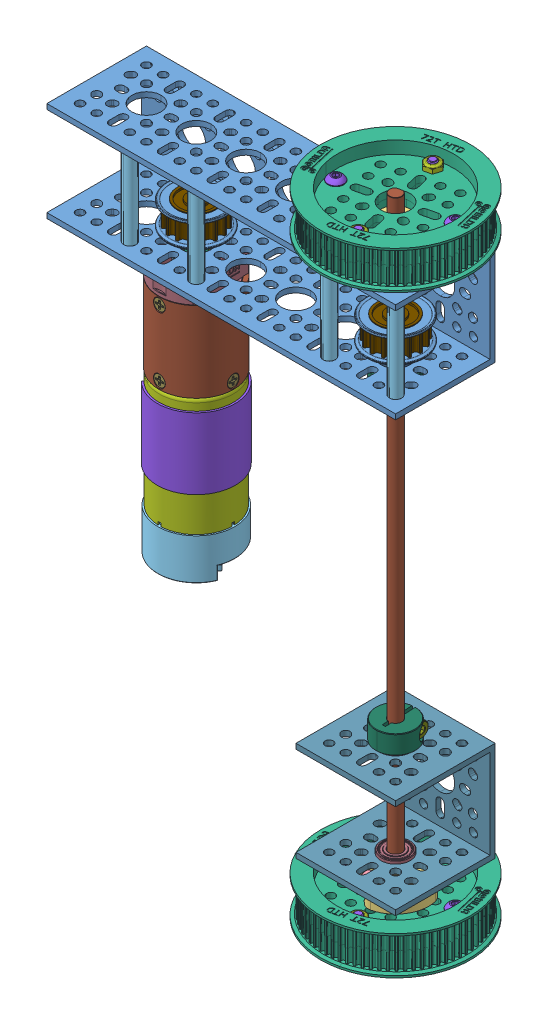
SolidWorks assembly motorisationElevateur, configuration Défaut. Lengths in mm.
Overall size (187.17 304.42 86.33).
106 component instances, 34 part files, 50 mates.
Components (placement in the parent):
- 1120-0006-0168 channel-1: 1120-0006-0168 channel [Défaut] at (77.0358 3.4821 146.5) x (0 -1 0) z (0 0 -1) size (48 168 48)
- 5202-2402-0051 moteur-1: 5202-2402-0051 moteur [Défaut] at (-54.0426 -130.9533 205.1707) x (0 0 1) z (-1 0 0) size (52.36 150.75 52.36)
  - 5202-2402-0051.step-1: 5202-2402-0051.step [Défaut] at origin size (52.36 150.75 52.36)
    - 5000-0002-0001.step-1: 5000-0002-0001.step [Défaut] at origin size (52.36 88.75 52.36)
      - 5000-0002-0001 encoder cap.step-1: 5000-0002-0001 encoder cap.step [Défaut] x (0 1 0) z (0 0 1) size (22.84 52.33 52.33)
        - JST-XH-4POS-VERT (1).step-1: JST-XH-4POS-VERT (1).step [Défaut] at (2.8 12.25 -75.95) x (1 0 0) z (0 0 -1) size (10.4 12.83 12.83)
          - Plastic (1).step-1: Plastic (1).step [Défaut] at (-6.1146 -33.6358 -52.1967) x (0 0.707107 0.707107) z (-1 0 0) size (12.4 5.75 7)
          - Pin (1).step-1: Pin (1).step [Défaut] at (-7.7146 -29.3225 -51.2067) x (0 0.707107 0.707107) z (-1 0 0) size (0.64 0.64 10)
          - Pin (1).step-2: Pin (1).step [Défaut] at (-7.7146 -34.6258 -56.51) x (0 0.707107 0.707107) z (-1 0 0) size (0.64 0.64 10)
          - Pin (1).step-3: Pin (1).step [Défaut] at (-7.7146 -32.858 -54.7423) x (0 0.707107 0.707107) z (-1 0 0) size (0.64 0.64 10)
          - Pin (1).step-4: Pin (1).step [Défaut] at (-7.7146 -31.0902 -52.9745) x (0 0.707107 0.707107) z (-1 0 0) size (0.64 0.64 10)
        - screw.step-1: screw.step [Défaut] at (-41.264 -8.1646 3.9905) x (0.882398 0 0.470504) z (0 -1 0) size (8.86 7.85 4.95)
          - 99461A915_Phillips Rounded Head Thread-Forming Screws (1).step-1: 99461A915_Phillips Rounded Head Thread-Forming Screws (1).step [Défaut] at (27.264 -14.6475 -49.347) x (-0.332697 -0.623949 0.707107) z (-0.882398 0.470504 0) size (3.5 3.5 7.4)
        - screw_1.step-1: screw_1.step [Défaut] at (-14.4172 7.3354 3.9905) x (0.882398 0 0.470504) z (0 -1 0) size (8.86 7.85 4.95)
          - 99461A915_Phillips Rounded Head Thread-Forming Screws (1).step-1: 99461A915_Phillips Rounded Head Thread-Forming Screws (1).step [Défaut] at (-10.5142 -28.4382 -25.8237) x (-0.332697 -0.623949 0.707107) z (-0.882398 0.470504 0) size (3.5 3.5 7.4)
        - endcap.step-1: endcap.step [Défaut] at (72.6354 37.1707 -11.0784) x (0 -0.707107 -0.707107) z (1 0 0) size (37 37 21.84)
        - base.step-1: base.step [Défaut] at (-55.8646 37.1707 -11.0784) x (0 -0.707107 -0.707107) z (-1 0 0) size (34.96 34.31 1)
      - 5000-0002-0001 body.step-1: 5000-0002-0001 body.step [Défaut] at (-37.1707 3.4854 -11.0784) size (35.61 61.8 35.61)
      - 5000-0002-0001 motor shield.step-1: 5000-0002-0001 motor shield.step [Défaut] at (-37.1707 54.6354 -11.0784) x (0.808104 0 -0.58904) z (0 -1 0) size (37.5 37.27 34.15)
      - 5000-0002-0001 motor shaft.step-1: 5000-0002-0001 motor shaft.step [Défaut] at (-37.1707 59.4854 -11.0784) size (3.14 12.45 3.14)
    - 5102-0024-0051.step-1: 5102-0024-0051.step [Défaut] at origin size (36 76.68 35.98)
      - 5102 Gearbox Base.step-1: 5102 Gearbox Base.step [Défaut] at (-37.1707 60.1354 -11.0784) size (31.91 5.69 31.91)
      - 5102 Gearbox Barrel (3 stage, simple)_Gear Blank.step-1: 5102 Gearbox Barrel (3 stage, simple)_Gear Blank.step [Défaut] at (-37.1707 111.8354 -11.0784) x (1 0 0) z (0 -1 0) size (35.98 35.98 38.7)
      - 5102 Gearbox Barrel Screw (M3 x 8mm length Flat Head)_92010A118.step-1: 5102 Gearbox Barrel Screw (M3 x 8mm length Flat Head)_92010A118.step [Défaut] at (-37.1707 63.6354 5.0046) x (0.002439 -0.999997 0) z (0 0 1) size (5.46 5.46 8)
      - 5102 Gearbox Face.step-1: 5102 Gearbox Face.step [Défaut] at (-37.1707 93.3354 -11.0784) size (36 17.1 31.91)
      - 5102 Gearbox Bearing.step-1: 5102 Gearbox Bearing.step [Défaut] at (-37.1707 101.4354 -11.0784) size (17 5 17)
      - 5102 Gearbox Shaft (23.5mm Length, Simple).step-1: 5102 Gearbox Shaft (23.5mm Length, Simple).step [Défaut] at (-37.1707 89.9754 -11.0784) x (0.894773 0 -0.44652) z (0.44652 0 0.894773) size (8.97 40.6 8.97)
      - 5102 Gearbox Snap Ring.step-1: 5102 Gearbox Snap Ring.step [Défaut] at (-37.1707 106.5104 -11.0784) x (0 1 0) z (0 0 1) size (0.85 13.06 10.66)
      - 5102 Gearbox Barrel Screw (M3 x 8mm length Flat Head)_92010A118.step-2: 5102 Gearbox Barrel Screw (M3 x 8mm length Flat Head)_92010A118.step [Défaut] at (-37.1707 95.3354 5.0046) x (-0.002439 -0.999997 0) z (0 0 1) size (5.46 5.46 8)
      - 5102 Gearbox Barrel Screw (M3 x 8mm length Flat Head)_92010A118.step-3: 5102 Gearbox Barrel Screw (M3 x 8mm length Flat Head)_92010A118.step [Défaut] at (-21.0877 63.6354 -11.0784) x (0 -0.999997 -0.002439) z (1 0 0) size (5.46 5.46 8)
      - 5102 Gearbox Barrel Screw (M3 x 8mm length Flat Head)_92010A118.step-4: 5102 Gearbox Barrel Screw (M3 x 8mm length Flat Head)_92010A118.step [Défaut] at (-37.1707 63.6354 -27.1614) x (-0.002439 -0.999997 0) z (0 0 -1) size (5.46 5.46 8)
      - 5102 Gearbox Barrel Screw (M3 x 8mm length Flat Head)_92010A118.step-5: 5102 Gearbox Barrel Screw (M3 x 8mm length Flat Head)_92010A118.step [Défaut] at (-53.2537 63.6354 -11.0784) x (0 -0.999997 0.002439) z (-1 0 0) size (5.46 5.46 8)
      - 5102 Gearbox Barrel Screw (M3 x 8mm length Flat Head)_92010A118.step-6: 5102 Gearbox Barrel Screw (M3 x 8mm length Flat Head)_92010A118.step [Défaut] at (-21.0877 95.3354 -11.0784) x (0 -0.999997 0.002439) z (1 0 0) size (5.46 5.46 8)
      - 5102 Gearbox Barrel Screw (M3 x 8mm length Flat Head)_92010A118.step-7: 5102 Gearbox Barrel Screw (M3 x 8mm length Flat Head)_92010A118.step [Défaut] at (-37.1707 95.3354 -27.1614) x (0.002439 -0.999997 0) z (0 0 -1) size (5.46 5.46 8)
      - 5102 Gearbox Barrel Screw (M3 x 8mm length Flat Head)_92010A118.step-8: 5102 Gearbox Barrel Screw (M3 x 8mm length Flat Head)_92010A118.step [Défaut] at (-53.2537 95.3354 -11.0784) x (0 -0.999997 -0.002439) z (-1 0 0) size (5.46 5.46 8)
      - 5102 Gearbox Bearing.step-2: 5102 Gearbox Bearing.step [Défaut] at (-37.1707 93.3354 -11.0784) size (17 5 17)
      - 5102 Gearbox Base Mounting Screw M3 x 5mm length SHCS)_91290A110.step-1: 5102 Gearbox Base Mounting Screw M3 x 5mm length SHCS)_91290A110.step [Défaut] at (-46.0096 57.2554 -2.2396) x (0.056382 0 0.998409) z (0 -1 0) size (5.5 5.5 8)
      - 5102 Gearbox Base Mounting Screw M3 x 5mm length SHCS)_91290A110.step-2: 5102 Gearbox Base Mounting Screw M3 x 5mm length SHCS)_91290A110.step [Défaut] at (-28.3319 57.2554 -2.2396) x (0.998409 0 -0.056382) z (0 -1 0) size (5.5 5.5 8)
      - 5102 Gearbox Base Mounting Screw M3 x 5mm length SHCS)_91290A110.step-3: 5102 Gearbox Base Mounting Screw M3 x 5mm length SHCS)_91290A110.step [Défaut] at (-28.3319 57.2554 -19.9173) x (-0.056382 0 -0.998409) z (0 -1 0) size (5.5 5.5 8)
      - 5102 Gearbox Base Mounting Screw M3 x 5mm length SHCS)_91290A110.step-4: 5102 Gearbox Base Mounting Screw M3 x 5mm length SHCS)_91290A110.step [Défaut] at (-46.0096 57.2554 -19.9173) x (-0.998409 0 0.056382) z (0 -1 0) size (5.5 5.5 8)
- 3417-1006-0016 assembly pulley-1: 3417-1006-0016 assembly pulley [Défaut] at (-65.9677 49.45 158.6429) x (0 1 0) z (1 0 0) size (12.01 27.98 27.98)
  - 3417-1006-0016 assembly.STEP-1: 3417-1006-0016 assembly.STEP [Défaut] at origin size (12.01 27.98 27.98)
    - 3417-1006-0016 body.STEP-1: 3417-1006-0016 body.STEP [Défaut] at (-62.7232 -4.1348 4.7756) size (12 23.97 23.97)
    - 3417-1006-0016 ring.STEP-1: 3417-1006-0016 ring.STEP [Défaut] at (-50.8429 9.3571 23.0035) x (0 -1 0) z (0 0 1) size (27.98 1.38 27.98)
    - 3417-1006-0016 ring.STEP-2: 3417-1006-0016 ring.STEP [Défaut] at (-60.0929 9.3571 23.0035) x (0 -1 0) z (0 0 -1) size (27.98 1.38 27.98)
    - 2806-0005-0006_91390A118.STEP-1: 2806-0005-0006_91390A118.STEP [Défaut] at (-55.4679 9.3571 17.1119) x (-0.607877 0.794031 0) z (0 0 -1) size (5.01 5.01 6.01)
- 3417-1006-0016 assembly pulley-2: 3417-1006-0016 assembly pulley [Défaut] at (56.9629 49.45 143.4787) x (0 1 0) z (0.225568 0 0.974227) size (12.01 27.98 27.98)
  - 3417-1006-0016 assembly.STEP-1: 3417-1006-0016 assembly.STEP [Défaut] at origin size (12.01 27.98 27.98)
    - 3417-1006-0016 body.STEP-1: 3417-1006-0016 body.STEP [Défaut] at (-62.7232 -4.1348 4.7756) size (12 23.97 23.97)
    - 3417-1006-0016 ring.STEP-1: 3417-1006-0016 ring.STEP [Défaut] at (-50.8429 9.3571 23.0035) x (0 -1 0) z (0 0 1) size (27.98 1.38 27.98)
    - 3417-1006-0016 ring.STEP-2: 3417-1006-0016 ring.STEP [Défaut] at (-60.0929 9.3571 23.0035) x (0 -1 0) z (0 0 -1) size (27.98 1.38 27.98)
    - 2806-0005-0006_91390A118.STEP-1: 2806-0005-0006_91390A118.STEP [Défaut] at (-55.4679 9.3571 17.1119) x (-0.607877 0.794031 0) z (0 0 -1) size (5.01 5.01 6.01)
- 1309-0016-1006 assembly-1: 1309-0016-1006 assembly [Défaut] at (37.2879 44.7557 158.8543) x (-0.848383 0 -0.529382) z (0 -1 0) size (28.36 32 10.95)
  - 1309-0016-1006 assembly.STEP-1: 1309-0016-1006 assembly.STEP [Défaut] at origin size (28.36 32 10.95)
    - 1309-0016-1006.STEP-1: 1309-0016-1006.STEP [Défaut] at (-18.2019 0.5776 8.7736) size (25.38 32 10)
    - 2800-0004-0014_90128A207.STEP-1: 2800-0004-0014_90128A207.STEP [Défaut] at (-16.149 11.6963 8.7736) x (0.5 -0.5 -0.707107) z (0.707107 0.707107 0) size (7 7 18.01)
    - 2800-0004-0014_90128A207.STEP-2: 2800-0004-0014_90128A207.STEP [Défaut] at (-20.2547 -10.5411 8.7736) x (-0.5 0.5 -0.707107) z (-0.707107 -0.707107 0) size (7 7 18.01)
- 1501-0006-0430 renfort-1: 1501-0006-0430 renfort [Défaut] at (69.0358 3.4821 184) size (5.95 43.01 5.95)
- 1501-0006-0430 renfort-2: 1501-0006-0430 renfort [Défaut] at (37.0358 3.4821 184) size (5.95 43.01 5.95)
- 1501-0006-0430 renfort-3: 1501-0006-0430 renfort [Défaut] at (-26.9642 3.4821 184) size (5.95 43.01 5.95)
- 1501-0006-0430 renfort-4: 1501-0006-0430 renfort [Défaut] at (-58.9642 3.4821 184) size (5.95 43.01 5.95)
- 3402-0014-0072 pulley-1: 3402-0014-0072 pulley [Défaut] at (-4.0352 74.1976 188.4845) x (-0.974227 0 0.225568) z (0 -1 0) size (71.96 71.96 18.5)
  - 3402-0014-0072 assembly.STEP-1: 3402-0014-0072 assembly.STEP [Défaut] at origin size (71.96 71.96 18.5)
    - 3402-0014-0072.STEP-1: 3402-0014-0072.STEP [Défaut] at (-60.2208 7.0832 38.7155) size (71.96 71.96 10.5)
    - 3402-0014-0072.STEP-2: 3402-0014-0072.STEP [Défaut] at (-60.2208 7.0832 23.2155) x (0 -1 0) z (0 0 -1) size (71.96 71.96 10.5)
    - 2812-0004-0007_90576A103.STEP-1: 2812-0004-0007_90576A103.STEP [Défaut] at (-60.2208 31.0832 29.7155) x (0.866025 0.5 0) z (-0.5 0.866025 0) size (7.02 4.86 8.1)
    - 2812-0004-0007_90576A103.STEP-2: 2812-0004-0007_90576A103.STEP [Défaut] at (-60.2208 -16.9168 29.7155) x (0 1 0) z (-1 0 0) size (7.02 4.86 8.1)
    - 2812-0004-0007_90576A103.STEP-3: 2812-0004-0007_90576A103.STEP [Défaut] at (-84.2208 7.0832 32.2155) x (0.5 0.866025 0) z (0.866025 -0.5 0) size (7.02 4.86 8.1)
    - 2812-0004-0007_90576A103.STEP-4: 2812-0004-0007_90576A103.STEP [Défaut] at (-36.2208 7.0832 32.2155) x (1 0 0) z (0 -1 0) size (7.02 4.86 8.1)
    - 2802-0004-0010_92095A480.STEP-1: 2802-0004-0010_92095A480.STEP [Défaut] at (-36.2208 7.0832 25.5155) x (-0.923728 -0.383049 0) z (0 0 -1) size (13.53 12.99 15.57)
    - 2802-0004-0010_92095A480.STEP-2: 2802-0004-0010_92095A480.STEP [Défaut] at (-84.2208 7.0832 25.5155) x (0.923728 0.383049 0) z (0 0 -1) size (13.53 12.99 15.57)
    - 2802-0004-0010_92095A480.STEP-3: 2802-0004-0010_92095A480.STEP [Défaut] at (-60.2208 31.0832 36.4155) size (13.53 12.99 15.57)
    - 2802-0004-0010_92095A480.STEP-4: 2802-0004-0010_92095A480.STEP [Défaut] at (-60.2208 -16.9168 36.4155) x (-1 0 0) z (0 0 1) size (13.53 12.99 15.57)
- 2801-0004-0008-rondelle-1: 2801-0004-0008-rondelle [Défaut] at (53.0358 29.9821 168) x (0.947224 0 -0.320572) z (0 -1 0) size (8 8 1)
- 1611-0514-0006 Roulement-2: 1611-0514-0006 Roulement [Défaut] at (53.0358 28.9821 168) x (0.985961 0 0.166976) z (0.166976 0 -0.985961) size (15 5 15)
- 2101-0006-0300-1: 2101-0006-0300 [Défaut] at (53.0358 -249.726 168) x (0.974227 0 -0.225568) z (0.225568 0 0.974227) size (6 300 5.5)
- 1309-0016-1006 assembly-2: 1309-0016-1006 assembly [Défaut] at (63.1616 -244.2077 152.8636) x (0.529382 0 -0.848383) z (0 1 0) size (28.36 32 10.95)
  - 1309-0016-1006 assembly.STEP-1: 1309-0016-1006 assembly.STEP [Défaut] at origin size (28.36 32 10.95)
    - 1309-0016-1006.STEP-1: 1309-0016-1006.STEP [Défaut] at (-18.2019 0.5776 8.7736) size (25.38 32 10)
    - 2800-0004-0014_90128A207.STEP-1: 2800-0004-0014_90128A207.STEP [Défaut] at (-16.149 11.6963 8.7736) x (0.5 -0.5 -0.707107) z (0.707107 0.707107 0) size (7 7 18.01)
    - 2800-0004-0014_90128A207.STEP-2: 2800-0004-0014_90128A207.STEP [Défaut] at (-20.2547 -10.5411 8.7736) x (-0.5 0.5 -0.707107) z (-0.707107 -0.707107 0) size (7 7 18.01)
- 2807-0609-1000-1: 2807-0609-1000 [Défaut] at (53.0358 -229.434 168) size (9 1 9)
- 1611-0514-0006-3: 1611-0514-0006 [Défaut] at (53.0358 -223.434 168) x (-0.972788 0 0.231697) z (0.231697 0 0.972788) size (15 5 15)
- 1120-0001-0048 u1-1: 1120-0001-0048 u1 [Défaut] at (77.0358 -203.434 146.5) x (0 -1 0) z (0 0 -1) size (48 48 48)
- 1611-0514-0006-4: 1611-0514-0006 [Défaut] at (53.0358 -183.434 168) x (0.99995 0 -0.010033) z (0.010033 0 0.99995) size (15 5 15)
- 2910-0919-0006 assembly collet-4: 2910-0919-0006 assembly collet [Défaut] at (21.0508 -173.9545 153.1256) x (-0.998275 0 0.058717) z (0.058717 0 0.998275) size (19 9.89 19.83)
  - 2910-0919-0006 assembly.STEP-1: 2910-0919-0006 assembly.STEP [Défaut] at origin size (19 9.89 19.83)
    - 2910-0919-0006.STEP-1: 2910-0919-0006.STEP [Défaut] at (-31.0565 -0.5204 16.7268) size (19 9.5 18.97)
    - 2800-0004-0010_90128A207.STEP-1: 2800-0004-0010_90128A207.STEP [Défaut] at (-24.2865 -0.5204 11.2868) x (0 -0.807243 -0.59022) z (1 0 0) size (7 7 14.01)
- 3402-0014-0072 pulley-2: 3402-0014-0072 pulley [Défaut] at (-4.0352 -211.7186 188.4845) x (-0.974227 0 0.225568) z (0 -1 0) size (71.96 71.96 18.5)
  - 3402-0014-0072 assembly.STEP-1: 3402-0014-0072 assembly.STEP [Défaut] at origin size (71.96 71.96 18.5)
    - 3402-0014-0072.STEP-1: 3402-0014-0072.STEP [Défaut] at (-60.2208 7.0832 38.7155) size (71.96 71.96 10.5)
    - 3402-0014-0072.STEP-2: 3402-0014-0072.STEP [Défaut] at (-60.2208 7.0832 23.2155) x (0 -1 0) z (0 0 -1) size (71.96 71.96 10.5)
    - 2812-0004-0007_90576A103.STEP-1: 2812-0004-0007_90576A103.STEP [Défaut] at (-60.2208 31.0832 29.7155) x (0.866025 0.5 0) z (-0.5 0.866025 0) size (7.02 4.86 8.1)
    - 2812-0004-0007_90576A103.STEP-2: 2812-0004-0007_90576A103.STEP [Défaut] at (-60.2208 -16.9168 29.7155) x (0 1 0) z (-1 0 0) size (7.02 4.86 8.1)
    - 2812-0004-0007_90576A103.STEP-3: 2812-0004-0007_90576A103.STEP [Défaut] at (-84.2208 7.0832 32.2155) x (0.5 0.866025 0) z (0.866025 -0.5 0) size (7.02 4.86 8.1)
    - 2812-0004-0007_90576A103.STEP-4: 2812-0004-0007_90576A103.STEP [Défaut] at (-36.2208 7.0832 32.2155) x (1 0 0) z (0 -1 0) size (7.02 4.86 8.1)
    - 2802-0004-0010_92095A480.STEP-1: 2802-0004-0010_92095A480.STEP [Défaut] at (-36.2208 7.0832 25.5155) x (-0.923728 -0.383049 0) z (0 0 -1) size (13.53 12.99 15.57)
    - 2802-0004-0010_92095A480.STEP-2: 2802-0004-0010_92095A480.STEP [Défaut] at (-84.2208 7.0832 25.5155) x (0.923728 0.383049 0) z (0 0 -1) size (13.53 12.99 15.57)
    - 2802-0004-0010_92095A480.STEP-3: 2802-0004-0010_92095A480.STEP [Défaut] at (-60.2208 31.0832 36.4155) size (13.53 12.99 15.57)
    - 2802-0004-0010_92095A480.STEP-4: 2802-0004-0010_92095A480.STEP [Défaut] at (-60.2208 -16.9168 36.4155) x (-1 0 0) z (0 0 1) size (13.53 12.99 15.57)
- 1611-0514-0006 Roulement-3: 1611-0514-0006 Roulement [Défaut] at (53.0358 -16.5179 168) x (1 0 0) z (0 0 -1) size (15 5 15)
- 2910-0919-0006 assembly collet-5: 2910-0919-0006 assembly collet [Défaut] at (84.0923 -25.9975 151.2732) size (19 9.89 19.83)
  - 2910-0919-0006 assembly.STEP-1: 2910-0919-0006 assembly.STEP [Défaut] at origin size (19 9.89 19.83)
    - 2910-0919-0006.STEP-1: 2910-0919-0006.STEP [Défaut] at (-31.0565 -0.5204 16.7268) size (19 9.5 18.97)
    - 2800-0004-0010_90128A207.STEP-1: 2800-0004-0010_90128A207.STEP [Défaut] at (-24.2865 -0.5204 11.2868) x (0 -0.807243 -0.59022) z (1 0 0) size (7 7 14.01)
Mates (geometry in assembly coordinates):
- Coaxiale1: concentric: cylinder of 5202-2402-0051 moteur-1/5202-2402-0051.step-1/5102-0024-0051.step-1/5102 Gearbox Shaft (23.5mm Length, Simple).step-1 through (-42.9642 -22.5179 168) axis (0 1 0) radius 3; cylinder of 1120-0006-0168 channel-1 through (-42.9642 -10.5179 168) axis (0 -1 0) radius 7
- Coïncidente1: coincident: plane of 1120-0006-0168 channel-1 through (-90.9642 -20.5179 192) normal (0 -1 0); plane of 5202-2402-0051 moteur-1/5202-2402-0051.step-1/5102-0024-0051.step-1/5102 Gearbox Face.step-1 through (-42.9642 -20.5179 168) normal (0 1 0)
- Coaxiale7: concentric: cylinder of 5202-2402-0051 moteur-1/5202-2402-0051.step-1/5102-0024-0051.step-1/5102 Gearbox Shaft (23.5mm Length, Simple).step-1 through (-42.9642 -22.5179 168) axis (0 1 0) radius 3; cylinder of 3417-1006-0016 assembly pulley-1/3417-1006-0016 assembly.STEP-1/3417-1006-0016 body.STEP-1 through (-42.9642 -22.648 168) axis (0 1 0) radius 3
- Parallèle2: parallel: plane of 5202-2402-0051 moteur-1/5202-2402-0051.step-1/5102-0024-0051.step-1/5102 Gearbox Shaft (23.5mm Length, Simple).step-1; line of 3417-1006-0016 assembly pulley-1/3417-1006-0016 assembly.STEP-1/3417-1006-0016 body.STEP-1 through (-45.2546 -0.0179 166.0625) axis (-0.104279 0 0.994548)
- Coaxiale8: concentric: cylinder of 1120-0006-0168 channel-1 through (53.0358 17.4821 168) axis (0 1 0) radius 7; cylinder of 3417-1006-0016 assembly pulley-2/3417-1006-0016 assembly.STEP-1/3417-1006-0016 body.STEP-1 through (53.0358 -22.648 168) axis (0 1 0) radius 3
- Coïncidente21: coincident: plane of 1120-0006-0168 channel-1 through (-90.9642 -18.0179 146.5) normal (0 1 0); plane of 1501-0006-0430 renfort-1 through (69.0358 -18.0179 184) normal (0 -1 0)
- Coïncidente22: coincident: plane of 1120-0006-0168 channel-1 through (-90.9642 -18.0179 146.5) normal (0 1 0); plane of 1501-0006-0430 renfort-2 through (37.0358 -18.0179 184) normal (0 -1 0)
- Coaxiale18: concentric: cylinder of 1120-0006-0168 channel-1 through (69.0358 -10.5179 184) axis (0 -1 0) radius 2; cylinder of 1501-0006-0430 renfort-1 through (69.0358 24.9821 184) axis (0 -1 0) radius 2.975
- Coaxiale19: concentric: circle of 1120-0006-0168 channel-1; cylinder of 1501-0006-0430 renfort-2 through (37.0358 24.9821 184) axis (0 -1 0) radius 2.975
- Coïncidente23: coincident: plane of 3417-1006-0016 assembly pulley-1/3417-1006-0016 assembly.STEP-1/3417-1006-0016 body.STEP-1 through (-37.7077 -0.0179 178.4916) normal (0 1 0); plane of 3417-1006-0016 assembly pulley-2/3417-1006-0016 assembly.STEP-1/3417-1006-0016 body.STEP-1 through (44.8303 -0.0179 176.389) normal (0 1 0)
- Coïncidente24: coincident: plane of 1120-0006-0168 channel-1 through (-90.9642 -18.0179 146.5) normal (0 1 0); plane of 1501-0006-0430 renfort-4 through (-50.9642 -18.0179 184) normal (0 -1 0)
- Coïncidente25: coincident: plane of 1120-0006-0168 channel-1 through (-90.9642 -18.0179 146.5) normal (0 1 0); plane of 1501-0006-0430 renfort-3 through (-82.9642 -18.0179 184) normal (0 -1 0)
- Coaxiale20: concentric: cylinder of 1501-0006-0430 renfort-3 through (-26.9642 24.9821 184) axis (0 -1 0) radius 2.975; cylinder of 1120-0006-0168 channel-1 through (-26.9642 -10.5179 184) axis (0 -1 0) radius 2
- Coaxiale21: concentric: cylinder of 1501-0006-0430 renfort-4 through (-58.9642 24.9821 184) axis (0 -1 0) radius 2.975; cylinder of 1120-0006-0168 channel-1 through (-58.9642 -10.5179 184) axis (0 -1 0) radius 2
- Coïncidente29: coincident: plane of 1309-0016-1006 assembly-1/1309-0016-1006 assembly.STEP-1/1309-0016-1006.STEP-1 through (53.0358 39.9821 168) normal (0 1 0); plane of 3402-0014-0072 pulley-1/3402-0014-0072 assembly.STEP-1/3402-0014-0072.STEP-2 through (53.0358 39.9821 168) normal (0 -1 0)
- Coaxiale25: concentric: circle of 1309-0016-1006 assembly-1/1309-0016-1006 assembly.STEP-1/1309-0016-1006.STEP-1; circle of 3402-0014-0072 pulley-1/3402-0014-0072 assembly.STEP-1/3402-0014-0072.STEP-1
- Coaxiale27: concentric: cylinder of 1120-0006-0168 channel-1 through (53.0358 17.4821 168) axis (0 1 0) radius 7; cylinder of 1611-0514-0006 Roulement-2 through (53.0358 24.9821 168) axis (0 1 0) radius 7
- Coïncidente31: coincident: plane of 1120-0006-0168 channel-1 through (-90.9642 24.9821 146.5) normal (0 -1 0); plane of 1611-0514-0006 Roulement-2 through (53.0358 24.9821 168) normal (0 1 0)
- Coaxiale28: concentric: cylinder of 2801-0004-0008-rondelle-1 through (53.0358 28.9821 168) axis (0 1 0) radius 2; cylinder of 1611-0514-0006 Roulement-2 through (53.0358 28.9821 168) axis (0 -1 0) radius 3
- Coïncidente32: coincident: plane of 2801-0004-0008-rondelle-1 through (53.0358 28.9821 168) normal (0 -1 0); plane of 1611-0514-0006 Roulement-2 through (53.0358 28.9821 168) normal (0 1 0)
- Coaxiale31: concentric: cylinder of 1309-0016-1006 assembly-1/1309-0016-1006 assembly.STEP-1/1309-0016-1006.STEP-1 through (53.0358 40.2326 168) axis (0 -1 0) radius 3; cylinder of 2801-0004-0008-rondelle-1 through (53.0358 28.9821 168) axis (0 1 0) radius 2
- Coaxiale32: concentric: cylinder of 1309-0016-1006 assembly-1/1309-0016-1006 assembly.STEP-1/1309-0016-1006.STEP-1 through (53.0358 40.2326 168) axis (0 -1 0) radius 3; cylinder of 3402-0014-0072 pulley-1/3402-0014-0072 assembly.STEP-1/3402-0014-0072.STEP-1 through (53.0358 39.2321 168) axis (0 1 0) radius 7
- Coïncidente34: coincident: plane of 1309-0016-1006 assembly-1/1309-0016-1006 assembly.STEP-1/1309-0016-1006.STEP-1 through (53.0358 29.9821 168) normal (0 -1 0); plane of 2801-0004-0008-rondelle-1 through (53.0358 29.9821 168) normal (0 1 0)
- Coïncidente35: coincident: plane of 3417-1006-0016 assembly pulley-2/3417-1006-0016 assembly.STEP-1/3417-1006-0016 body.STEP-1 through (65.6206 -22.648 162.5406) normal (0.225568 0 0.974227); plane of 1309-0016-1006 assembly-1/1309-0016-1006 assembly.STEP-1/1309-0016-1006.STEP-1 through (52.4764 40.2326 165.5839) normal (0.225568 0 0.974227)
- Coaxiale33: concentric: cylinder of 1309-0016-1006 assembly-1/1309-0016-1006 assembly.STEP-1/1309-0016-1006.STEP-1 through (53.0358 40.2326 168) axis (0 -1 0) radius 3; cylinder of 2101-0006-0300-1 through (53.0358 50.274 168) axis (0 -1 0) radius 3
- Parallèle5: parallel: plane of 1309-0016-1006 assembly-1/1309-0016-1006 assembly.STEP-1/1309-0016-1006.STEP-1 through (52.4764 40.2326 165.5839) normal (0.225568 0 0.974227); plane of 2101-0006-0300-1 through (52.4719 50.274 165.5644) normal (-0.225568 0 -0.974227)
- Distance2: distance = 10.2919 mm: plane of 1309-0016-1006 assembly-1/1309-0016-1006 assembly.STEP-1/1309-0016-1006.STEP-1 through (53.0358 39.9821 168) normal (0 1 0); plane of 2101-0006-0300-1 through (53.0358 50.274 168) normal (0 1 0)
- Coaxiale34: concentric: cylinder of 2101-0006-0300-1 through (53.0358 50.274 168) axis (0 -1 0) radius 3; cylinder of 1309-0016-1006 assembly-2/1309-0016-1006 assembly.STEP-1/1309-0016-1006.STEP-1 through (53.0358 -239.6845 168) axis (0 1 0) radius 3
- Parallèle6: parallel: plane of 2101-0006-0300-1 through (52.4719 50.274 165.5644) normal (-0.225568 0 -0.974227); plane of 1309-0016-1006 assembly-2/1309-0016-1006 assembly.STEP-1/1309-0016-1006.STEP-1 through (52.4764 -239.6845 165.5839) normal (0.225568 0 0.974227)
- Distance3: distance = 10.2919 mm: plane of 2101-0006-0300-1 through (53.0358 -249.726 168) normal (0 -1 0); plane of 1309-0016-1006 assembly-2/1309-0016-1006 assembly.STEP-1/1309-0016-1006.STEP-1 through (53.0358 -239.434 168) normal (0 -1 0)
- Coaxiale35: concentric: cylinder of 2101-0006-0300-1 through (53.0358 50.274 168) axis (0 -1 0) radius 3; cylinder of 2807-0609-1000-1 through (53.0358 -228.434 168) axis (0 -1 0) radius 3
- Coïncidente40: coincident: plane of 1309-0016-1006 assembly-2/1309-0016-1006 assembly.STEP-1/1309-0016-1006.STEP-1 through (53.0358 -229.434 168) normal (0 1 0); plane of 2807-0609-1000-1 through (53.0358 -229.434 168) normal (0 -1 0)
- Coaxiale36: concentric: cylinder of 2101-0006-0300-1 through (53.0358 50.274 168) axis (0 -1 0) radius 3; cylinder of 1611-0514-0006-3 through (53.0358 -223.434 168) axis (0 -1 0) radius 3
- Coïncidente41: coincident: plane of 2807-0609-1000-1 through (53.0358 -228.434 168) normal (0 1 0); plane of 1611-0514-0006-3 through (53.0358 -228.434 168) normal (0 -1 0)
- Coaxiale37: concentric: cylinder of 1611-0514-0006-3 through (53.0358 -227.434 168) axis (0 1 0) radius 7; cylinder of 1120-0001-0048 u1-1 through (53.0358 -217.434 168) axis (0 -1 0) radius 7
- Coïncidente42: coincident: plane of 1611-0514-0006-3 through (53.0358 -227.434 168) normal (0 1 0); plane of 1120-0001-0048 u1-1 through (29.0358 -227.434 192) normal (0 -1 0)
- Coïncidente43: coincident: plane of 1120-0006-0168 channel-1 through (-90.9642 -20.5179 144) normal (0 0 -1); plane of 1120-0001-0048 u1-1 through (29.0358 -227.434 144) normal (0 0 -1)
- Coaxiale38: concentric: cylinder of 1120-0001-0048 u1-1 through (53.0358 -189.434 168) axis (0 1 0) radius 7; cylinder of 1611-0514-0006-4 through (53.0358 -179.434 168) axis (0 -1 0) radius 7
- Coïncidente44: coincident: plane of 1120-0001-0048 u1-1 through (29.0358 -179.434 192) normal (0 1 0); plane of 1611-0514-0006-4 through (53.0358 -179.434 168) normal (0 -1 0)
- Coaxiale40: concentric: cylinder of 2101-0006-0300-1 through (53.0358 50.274 168) axis (0 -1 0) radius 3; cylinder of 2910-0919-0006 assembly collet-4/2910-0919-0006 assembly.STEP-1/2910-0919-0006.STEP-1 through (53.0358 -177.934 168) axis (0 1 0) radius 3
- Coaxiale41: concentric: cylinder of 2101-0006-0300-1 through (53.0358 50.274 168) axis (0 -1 0) radius 3; cylinder of 3402-0014-0072 pulley-2/3402-0014-0072 assembly.STEP-1/3402-0014-0072.STEP-1 through (53.0358 -246.684 168) axis (0 1 0) radius 7
- Coïncidente46: coincident: plane of 1309-0016-1006 assembly-2/1309-0016-1006 assembly.STEP-1/1309-0016-1006.STEP-1 through (53.0358 -239.434 168) normal (0 -1 0); plane of 3402-0014-0072 pulley-2/3402-0014-0072 assembly.STEP-1/3402-0014-0072.STEP-1 through (53.0358 -239.434 168) normal (0 1 0)
- Coaxiale42: concentric: circle of 1309-0016-1006 assembly-2/1309-0016-1006 assembly.STEP-1/1309-0016-1006.STEP-1; circle of 3402-0014-0072 pulley-2/3402-0014-0072 assembly.STEP-1/3402-0014-0072.STEP-2
- Coïncidente48: coincident: plane of 1611-0514-0006-4 through (53.0358 -178.434 168) normal (0 1 0); plane of 2910-0919-0006 assembly collet-4/2910-0919-0006 assembly.STEP-1/2910-0919-0006.STEP-1 through (53.0358 -178.434 168) normal (0 -1 0)
- Coaxiale44: concentric: cylinder of 2101-0006-0300-1 through (53.0358 50.274 168) axis (0 -1 0) radius 3; cylinder of 1611-0514-0006 Roulement-3 through (53.0358 -16.5179 168) axis (0 -1 0) radius 3
- Coïncidente50: coincident: plane of 1120-0006-0168 channel-1 through (-90.9642 -20.5179 192) normal (0 -1 0); plane of 1611-0514-0006 Roulement-3 through (53.0358 -20.5179 168) normal (0 1 0)
- Coaxiale45: concentric: cylinder of 2101-0006-0300-1 through (53.0358 50.274 168) axis (0 -1 0) radius 3; cylinder of 2910-0919-0006 assembly collet-5/2910-0919-0006 assembly.STEP-1/2910-0919-0006.STEP-1 through (53.0358 -22.0179 168) axis (0 -1 0) radius 3
- Coïncidente51: coincident: plane of 1611-0514-0006 Roulement-3 through (53.0358 -21.5179 168) normal (0 -1 0); plane of 2910-0919-0006 assembly collet-5/2910-0919-0006 assembly.STEP-1/2910-0919-0006.STEP-1 through (53.0358 -21.5179 168) normal (0 1 0)
- Distance4: distance = 3 mm: plane of 3417-1006-0016 assembly pulley-1/3417-1006-0016 assembly.STEP-1/3417-1006-0016 body.STEP-1 through (-36.6423 -0.0179 177.8863) normal (0 1 0); plane of 5202-2402-0051 moteur-1/5202-2402-0051.step-1/5102-0024-0051.step-1/5102 Gearbox Shaft (23.5mm Length, Simple).step-1 through (-42.9642 2.9821 168) normal (0 1 0)
- Coaxiale46: concentric: circle of 1120-0006-0168 channel-1; circle of 5202-2402-0051 moteur-1/5202-2402-0051.step-1/5102-0024-0051.step-1/5102 Gearbox Face.step-1
